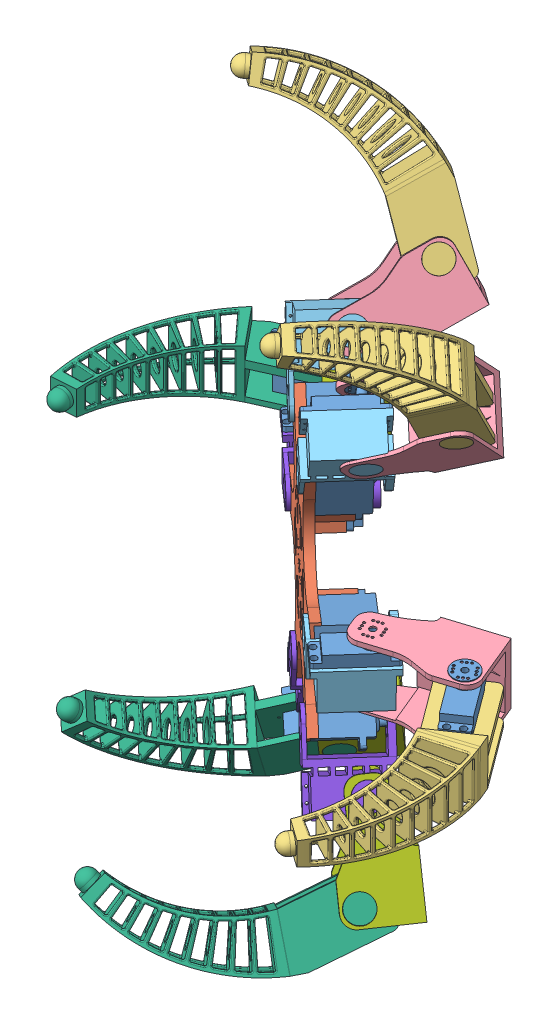
SolidWorks assembly hexa, configuration Default. Lengths in mm.
Overall size (514.39 542.6 425.45).
37 component instances, 8 part files, 28 mates.
Components (placement in the parent):
- 001-1: 001 [Default] at (-19.6958 -3.9572 43.3954) x (0.911676 0 -0.41091) z (0.41091 0 0.911676) size (54 47.2 20)
- 222-1: 222 [Default] at (118.7093 20.2009 195.5008) x (0.270581 0.932138 0.240633) z (-0.696541 0.362103 -0.619446) size (207.02 30.8 191.28)
- L1-1: L1 [Default] at (337.5516 24.6542 404.5688) x (0.063216 0.996415 0.056219) z (-0.991779 0.069002 -0.107767) size (43.78 187.09 90.57)
- L2-1: L2 [Default] at (240.9301 40.7962 284.926) x (-0.063216 -0.996415 -0.056219) z (0.344681 -0.074663 0.935746) size (53.5 90 50)
- L3-1: L3 [Default] at (239.3328 48.7526 265.771) x (-0.744572 0.084597 -0.66216) z (-0.063216 -0.996415 -0.056219) size (68.1 55.2 33)
- R1-1: R1 [Default] at (-113.4582 14.0428 162.755) x (0.918269 0 0.395956) z (0.395956 0 -0.918269) size (90.72 43.97 186.99)
- R2-1: R2 [Default] at (34.9688 21.4428 103.7331) x (0 1 0) z (-0.719377 0 0.69462) size (53.5 90 50)
- R3-1: R3 [Default] at (35.8243 -4.0572 84.8544) x (-0.664543 0 0.74725) z (0 1 0) size (55.2 68.1 33)
- 001-2: 001 [Default] at (60.8915 7.4676 136.3207) x (-0.738513 -0.152479 -0.656772) z (0.11394 -0.988307 0.101329) size (54 47.2 20)
- 001-3: 001 [Default] at (35.8949 -4.0572 84.8502) x (0.664543 0 -0.74725) z (0.74725 0 0.664543) size (54 47.2 20)
- 001-4: 001 [Default] at (237.4923 20.8572 264.2012) x (0.664543 0 -0.74725) z (0.744572 -0.084597 0.66216) size (54 47.2 20)
- 001-5: 001 [Default] at (314.4412 18.5763 253.6775) x (-0.578978 0.082498 -0.811159) z (0.812889 -0.018728 -0.582118) size (54 47.2 20)
- 001-7: 001 [Default] at (184.2357 32.9342 246.0128) x (0.738513 0.152479 0.656772) z (-0.11394 0.988307 -0.101329) size (54 47.2 20)
- 001-8: 001 [Default] at (99.9678 -57.6406 171.0719) x (-0.270581 -0.932138 -0.240633) z (0.696541 -0.362103 0.619446) size (54 47.2 20)
- 001-9: 001 [Default] at (161.6399 -44.9073 225.9179) x (0.467931 -0.779659 0.416139) z (0.582601 0.626204 0.518117) size (54 47.2 20)
- R3-2: R3 [Default] at (102.1358 -109.2444 143.8263) x (-0.664543 0 0.74725) z (-0.647138 0.5 -0.575511) size (55.2 68.1 33)
- R3-3: R3 [Default] at (203.3622 -84.9863 233.8486) x (-0.664543 0 0.74725) z (-0.647138 -0.5 -0.575511) size (55.2 68.1 33)
- 001-10: 001 [Default] at (102.1877 -109.2011 143.8056) x (0.664543 0 -0.74725) z (0.373625 0.866025 0.332271) size (54 47.2 20)
- 001-11: 001 [Default] at (203.3767 -84.943 233.7947) x (0.664543 0 -0.74725) z (-0.373625 0.866025 -0.332271) size (54 47.2 20)
- R2-2: R2 [Default] at (80.3297 -86.1831 144.0734) x (-0.647138 0.5 -0.575511) z (-0.691 -0.065775 0.719856) size (53.5 90 50)
- R2-3: R2 [Default] at (172.659 -87.425 226.1834) x (-0.647138 -0.5 -0.575511) z (-0.634246 -0.065775 0.770328) size (53.5 90 50)
- 001-12: 001 [Default] at (72.3456 -168.9836 125.2494) x (0.759168 0.353497 -0.546538) z (0.069828 0.790595 0.608345) size (54 47.2 20)
- 001-13: 001 [Default] at (225.1611 -144.8255 261.1508) x (0.454153 0.353497 -0.817793) z (-0.612337 0.790595 0.001684) size (54 47.2 20)
- R1-2: R1 [Default] at (-36.5234 -151.968 231.1744) x (0.563584 0.822124 0.080529) z (0.513406 -0.272236 -0.81382) size (90.72 43.97 186.99)
- R1-3: R1 [Default] at (109.3759 -145.8099 360.9252) x (-0.145786 0.822124 -0.550326) z (0.748304 -0.272236 -0.60492) size (90.72 43.97 186.99)
- 001-14: 001 [Default] at (145.1595 98.0424 211.2616) x (0.270581 0.932138 0.240633) z (-0.696541 0.362103 -0.619446) size (54 47.2 20)
- 001-15: 001 [Default] at (83.4874 85.3091 156.4156) x (-0.467931 0.779659 -0.416139) z (-0.582601 -0.626204 -0.518117) size (54 47.2 20)
- L3-2: L3 [Default] at (169.7315 152.9781 203.8734) x (-0.427032 -0.820622 -0.379767) z (0.61321 -0.571471 0.545338) size (68.1 55.2 33)
- L3-3: L3 [Default] at (67.4826 124.4264 112.9417) x (0.31754 -0.90522 0.282393) z (0.676426 0.424944 0.601557) size (68.1 55.2 33)
- 001-16: 001 [Default] at (186.8468 136.9358 219.1612) x (0.664543 0 -0.74725) z (0.427032 0.820622 0.379767) size (54 47.2 20)
- 001-17: 001 [Default] at (86.4051 136.2796 129.8368) x (0.664543 0 -0.74725) z (-0.31754 0.90522 -0.282393) size (54 47.2 20)
- 001-18: 001 [Default] at (246.4012 179.5354 193.1684) x (-0.269317 -0.80026 -0.535772) z (0.742591 0.181672 -0.644635) size (54 47.2 20)
- 001-19: 001 [Default] at (108.2184 181.1601 70.2801) x (0.456779 -0.882758 0.109958) z (0.577755 0.2004 -0.791226) size (54 47.2 20)
- L1-2: L1 [Default] at (221.6613 284.3696 301.5056) x (-0.61321 0.571471 -0.545338) z (-0.732778 -0.669338 0.122566) size (43.78 187.09 90.57)
- L1-3: L1 [Default] at (-4.3555 279.9163 100.505) x (-0.676426 -0.424944 -0.601557) z (-0.125471 -0.73834 0.662655) size (43.78 187.09 90.57)
- L2-2: L2 [Default] at (171.2757 161.0574 222.9812) x (0.61321 -0.571471 0.545338) z (0.06443 0.724256 0.686514) size (53.5 90 50)
- L2-3: L2 [Default] at (58.6229 140.4621 122.7972) x (0.676426 0.424944 0.601557) z (-0.592706 0.798919 0.102111) size (53.5 90 50)
Mates (geometry in assembly coordinates):
- Coincident2: coincident anti-aligned: plane of 001-1 through (-33.8202 34.0428 60.7304) normal (0.41091 0 0.911676); plane of R1-1 through (2.738 12.6428 44.2529) normal (-0.41091 0 -0.911676)
- Coincident3: coincident anti-aligned: plane of 001-1 through (-42.0384 34.0428 42.4968) normal (-0.911676 0 0.41091); plane of R1-1 through (-42.0795 12.6428 42.4057) normal (0.911676 0 -0.41091)
- Coincident4: coincident anti-aligned: plane of 001-1 through (-10.5791 43.2428 39.2863) normal (0 1 0); plane of R2-1 through (-10.5791 43.2428 39.2863) normal (0 -1 0)
- Concentric1: concentric anti-aligned: cylinder of 001-1 through (-10.5791 37.2428 39.2863) axis (0 1 0) radius 2.5; cylinder of R2-1 through (-10.5791 65.2428 39.2863) axis (0 -1 0) radius 2.5
- Coincident17: coincident anti-aligned: plane of 222-1 through (71.8074 10.5172 153.7902) normal (-0.738513 -0.152479 -0.656772); plane of 001-2 through (99.775 20.4003 120.0473) normal (0.738513 0.152479 0.656772)
- Coincident18: coincident anti-aligned: plane of 222-1 through (78.3739 20.4003 144.112) normal (0.11394 -0.988307 0.101329); plane of 001-2 through (99.775 20.4003 120.0473) normal (-0.11394 0.988307 -0.101329)
- Coincident19: coincident anti-aligned: plane of 222-1 through (141.1708 20.2009 170.2437) normal (0.664543 0 -0.74725); plane of 001-2 through (60.6983 -6.5324 98.6781) normal (-0.664543 0 0.74725)
- Coincident20: coincident anti-aligned: plane of 222-1 through (120.7029 20.2009 193.259) normal (-0.664543 0 0.74725); plane of R3-1 through (36.7007 36.1428 118.5544) normal (0.664543 0 -0.74725)
- Coincident21: coincident anti-aligned: plane of R3-1 through (56.6582 23.9428 76.5506) normal (-0.74725 0 -0.664543); plane of 001-3 through (30.0765 33.9428 106.4407) normal (0.74725 0 0.664543)
- Coincident22: coincident anti-aligned: plane of R3-1 through (35.8243 -4.0572 84.8544) normal (0 1 0); plane of 001-3 through (35.8949 -4.0572 84.8502) normal (0 -1 0)
- Coincident23: coincident anti-aligned: plane of R3-1 through (56.6582 23.9428 76.5506) normal (-0.664543 0 0.74725); plane of 001-3 through (41.7132 33.9428 63.2598) normal (0.664543 0 -0.74725)
- Concentric10: concentric anti-aligned: cylinder of R2-1 through (42.5029 3.7428 77.3445) axis (0 -1 0) radius 10.1; cylinder of R3-1 through (42.5029 -9.0572 77.3445) axis (0 1 0) radius 10
- Coincident24: coincident anti-aligned: plane of R2-1 through (70.9376 -7.0572 69.0022) normal (0 1 0); plane of R3-1 through (35.8243 -7.0572 84.8544) normal (0 -1 0)
- Coincident25: coincident anti-aligned: plane of L1-1 through (295.0541 26.4002 243.5317) normal (0.812889 -0.018728 -0.582118); plane of 001-5 through (320.294 54.9773 277.8581) normal (-0.812889 0.018728 0.582118)
- Coincident26: coincident anti-aligned: plane of L1-1 through (274.9747 21.3597 248.7214) normal (0.063216 0.996415 0.056219); plane of 001-5 through (314.4412 18.5763 253.6775) normal (-0.063216 -0.996415 -0.056219)
- Coincident27: coincident anti-aligned: plane of L1-1 through (318.2711 23.0921 276.0591) normal (-0.578978 0.082498 -0.811159); plane of 001-5 through (320.294 54.9773 277.8581) normal (0.578978 -0.082498 0.811159)
- Concentric11: concentric aligned: cylinder of L1-1 through (308.1884 12.4337 245.0644) axis (0.063216 0.996415 0.056219) radius 10; cylinder of L2-1 through (307.5689 2.6688 244.5135) axis (0.063216 0.996415 0.056219) radius 10.025
- Coincident28: coincident anti-aligned: plane of L1-1 through (377.0063 2.4937 397.2214) normal (-0.063216 -0.996415 -0.056219); plane of L2-1 through (309.2767 17.1855 212.9827) normal (0.063216 0.996415 0.056219)
- Coincident29: coincident anti-aligned: plane of L3-1 through (243.2143 18.7139 242.3912) normal (0.744572 -0.084597 0.66216); plane of 001-4 through (219.1579 59.5669 274.6609) normal (-0.744572 0.084597 -0.66216)
- Coincident30: coincident anti-aligned: plane of L3-1 through (231.532 17.0135 285.6653) normal (0.664543 0 -0.74725); plane of 001-4 through (219.1579 59.5669 274.6609) normal (-0.664543 0 0.74725)
- Coincident31: coincident anti-aligned: plane of L3-1 through (237.5628 20.8529 264.1969) normal (0.063216 0.996415 0.056219); plane of 001-4 through (237.4923 20.8572 264.2012) normal (-0.063216 -0.996415 -0.056219)
- Coincident32: coincident anti-aligned: plane of 222-1 through (174.4564 20.0016 229.5598) normal (-0.11394 0.988307 -0.101329); plane of 001-7 through (195.8575 20.0016 205.4951) normal (0.11394 -0.988307 0.101329)
- Coincident33: coincident anti-aligned: plane of 222-1 through (165.6111 29.8846 237.2114) normal (0.738513 0.152479 0.656772); plane of 001-7 through (195.8575 20.0016 205.4951) normal (-0.738513 -0.152479 -0.656772)
- Coincident34: coincident anti-aligned: plane of 222-1 through (168.3261 39.7677 231.8641) normal (0.664543 0 -0.74725); plane of 001-7 through (184.2357 32.9342 246.0128) normal (-0.664543 0 0.74725)
- Coincident35: coincident anti-aligned: plane of 222-1 through (120.7029 20.2009 193.259) normal (-0.664543 0 0.74725); plane of L3-1 through (202.7425 2.6753 266.2182) normal (0.664543 0 -0.74725)
- Concentric13: concentric aligned: cylinder of L2-1 through (243.3431 6.1018 255.8881) axis (0.063216 0.996415 0.056219) radius 10.025; cylinder of L3-1 through (243.9626 15.8666 256.439) axis (0.063216 0.996415 0.056219) radius 10
- Coincident36: coincident anti-aligned: plane of L2-1 through (222.163 20.3663 236.7754) normal (0.063216 0.996415 0.056219); plane of L3-1 through (237.3731 17.8637 264.0282) normal (-0.063216 -0.996415 -0.056219)
- Coincident37: coincident anti-aligned: plane of 001-1 through (9.0285 24.0428 41.4176) normal (0 -1 0); plane of R1-1 through (-79.1747 24.0428 29.2894) normal (0 1 0)
